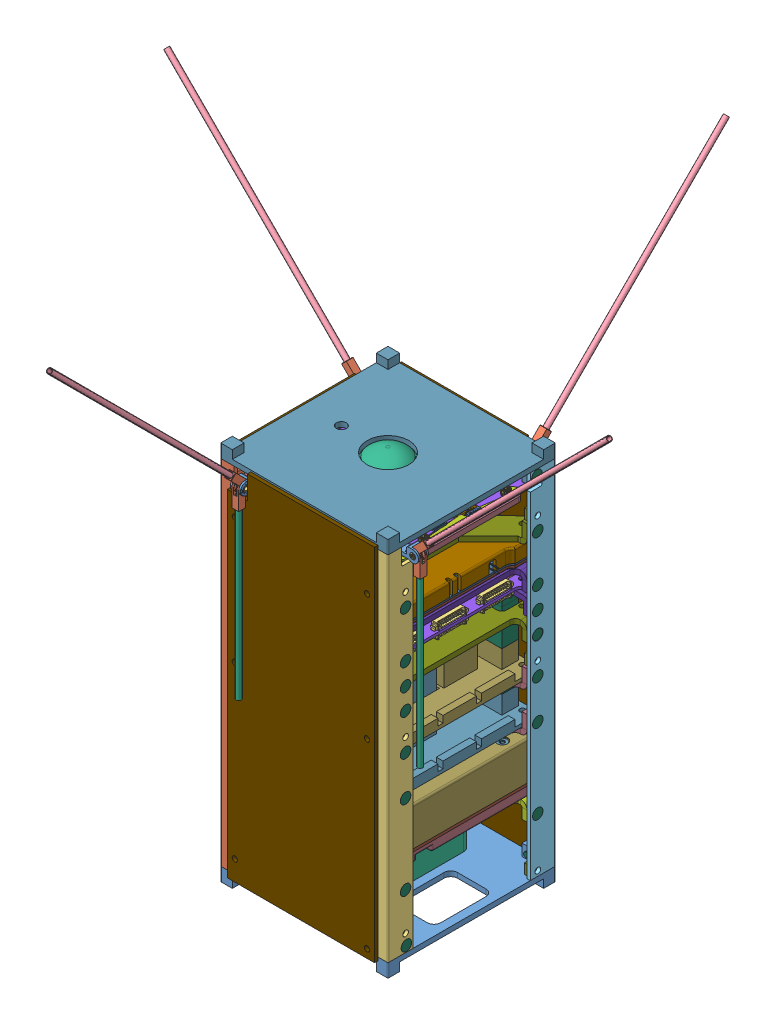
SolidWorks assembly Cubesat, configuration Default. Lengths in mm.
Overall size (336.69 331.47 336.69).
234 component instances, 66 part files, 161 mates.
Components (placement in the parent):
- Cover Plate Bottom-1: Cover Plate Bottom [Default] x (-1 0 0) z (0 0 1) size (100 15 100)
- Rail - Bottom Left-1: Rail - Bottom Left [Default] at (-50 0 50) size (15 211 15)
- Rail - Bottom Right-1: Rail - Bottom Right [Default] at (50 0 50) size (15 211 15)
- Rail - Top Left-1: Rail - Top Left [Default] at (-50 0 -35) size (15 211 15)
- Rail - Top Right-1: Rail - Top Right [Default] at (35 0 -35) size (15 211 15)
- Camera-1: Camera [Default] at (0 36.32 0) x (0 0 1) z (1 0 0) size (50.56 42.32 50.56)
- Camera Plate - 4 tabs - bottom-1: Camera Plate - 4 tabs - bottom [Default] at (0 39.32 0) size (96 10 96)
- EPS1+-1: EPS1+ [Default] at (47.8023 -33.6732 25.0624) x (0 0 -1) z (0 1 0) size (95.9 90.21 30)
  - EPS1+.STEP-1: EPS1+.STEP [Default] at origin size (95.9 90.21 30)
    - ESQ_126_69_G_D.STEP-1: ESQ_126_69_G_D.STEP [Default] at (61.6205 47.1532 90.3532) x (0 -1 0) z (-1 0 0) size (66.55 23.24 5.08)
      - _ESQ_126_69_G_D_socket_2.STEP-1: _ESQ_126_69_G_D_socket_2.STEP [Default] at (-33.274 0 0) size (66.55 8.51 4.95)
      - _ESQ_126_69_G_D_pins_4.STEP-1: _ESQ_126_69_G_D_pins_4.STEP [Default] at origin size (65.79 19.68 4.7)
      - _ESQ_126_69_G_D_LL_bpins_6.STEP-1: _ESQ_126_69_G_D_LL_bpins_6.STEP [Default] at (-33.147 -10.16 0) size (66.04 10.16 5.08)
    - ESQ_126_69_G_D.STEP-2: ESQ_126_69_G_D.STEP [Default] at (66.637 47.1532 90.3532) x (0 1 0) z (1 0 0) size (66.55 23.24 5.08)
      - _ESQ_126_69_G_D_socket_2.STEP-1: _ESQ_126_69_G_D_socket_2.STEP [Default] at (-33.274 0 0) size (66.55 8.51 4.95)
      - _ESQ_126_69_G_D_pins_4.STEP-1: _ESQ_126_69_G_D_pins_4.STEP [Default] at origin size (65.79 19.68 4.7)
      - _ESQ_126_69_G_D_LL_bpins_6.STEP-1: _ESQ_126_69_G_D_LL_bpins_6.STEP [Default] at (-33.147 -10.16 0) size (66.04 10.16 5.08)
    - ES_EPS_Rev1_4_PCB_STEP.STEP-1: ES_EPS_Rev1_4_PCB_STEP.STEP [Default] at (-22.8876 2.7023 80.1932) size (95.9 90.21 13.97)
    - top-cover.STEP-1: top-cover.STEP [Default] at (-22.8876 2.7023 80.1932) size (95.9 90.2 22.8)
    - bottom-cover_Rev1.2.STEP-1: bottom-cover_Rev1.2.STEP [Default] at (25.0624 47.8023 72.9932) size (95.9 90.2 13.5)
    - 965 M3x6 Torx_M3X6mm.STEP-1: 965 M3x6 Torx_M3X6mm.STEP [Default] at (54.8324 9.3023 102.3047) x (-0.142927 0.989733 0) z (0 0 1) size (5.5 5.5 6)
    - 965 M3x6 Torx_M3X6mm.STEP-2: 965 M3x6 Torx_M3X6mm.STEP [Default] at (54.8324 77.0023 102.394) x (0.179192 -0.983814 0) z (0 0 1) size (5.5 5.5 6)
    - TR Fastenings Ltd-M2_5X4mm.STEP-1: TR Fastenings Ltd-M2_5X4mm.STEP [Default] at (-22.8876 68.8523 83.4832) x (0 0.503629 0.86392) z (-1 0 0) size (4.7 4.7 4)
    - TR Fastenings Ltd-M2_5X4mm.STEP-2: TR Fastenings Ltd-M2_5X4mm.STEP [Default] at (-22.8876 26.7523 83.4832) x (0 -0.360323 0.932827) z (-1 0 0) size (4.7 4.7 4)
- Camera-2: Camera [Default] at (0 174.68 0) x (0 0 -1) z (1 0 0) size (50.56 42.32 50.56)
- Camera Plate - 4 tabs - top-1: Camera Plate - 4 tabs - top [Default] at (0 174.68 0) size (96 12 96)
- OBC_EnduroSat-1: OBC_EnduroSat [Default] at (44.1 146.28 47.95) x (0 0 -1) z (0 1 0) size (95 89.38 23.24)
  - OBC_EnduroSat.STEP-1: OBC_EnduroSat.STEP [Default] at origin size (95 89.38 23.24)
    - SD1021117.STEP-1: SD1021117.STEP [Default] at origin size (15.2 14.1 1.88)
      - User_Library-473521001_microSD.STEP-1: User_Library-473521001_microSD.STEP [Default] at (11.4631 39.834 0.9) x (0 -1 0) z (0 0 1) size (14.1 15.2 1.88)
    - P1021117.STEP-1: P1021117.STEP [Default] at origin size (10.15 5.2 3.4)
      - MOLEX_Pico_Blade_532610471.STEP-1: MOLEX_Pico_Blade_532610471.STEP [Default] at (43.8404 79.9325 1.7) size (10.15 5.2 3.4)
        - Open CASCADE STEP translator 6.8 1.14.1.1.STEP-1: Open CASCADE STEP translator 6.8 1.14.1.1.STEP [Default] at origin size (10.15 5.2 3.4)
    - USB1021117.STEP-1: USB1021117.STEP [Default] at origin size (9.9 9.22 5.09)
      - USB_Mini_B_SMT_Horisontal.STEP-1: USB_Mini_B_SMT_Horisontal.STEP [Default] at (43.8628 84.9308 -3.6122) x (1 0 0) z (0 1 0) size (9.9 5.09 9.22)
    - U1021117.STEP-1: U1021117.STEP [Default] at origin size (25.77 25.77 1.57)
      - User_Library-LQFP176-0_5.STEP-1: User_Library-LQFP176-0_5.STEP [Default] at (45.653 34.1752 0.75) x (1 0 0) z (0 0 1) size (25.77 25.77 1.57)
    - PAN6021117.STEP-1: PAN6021117.STEP [Default] at origin size (20.15 5.2 3.5)
      - MOLEX_Pico_Blade_532611271.STEP-1: MOLEX_Pico_Blade_532611271.STEP [Default] at (74.0242 8.708 -1.6) x (-1 0 0) z (0 0 -1) size (20.15 5.2 3.5)
    - PAN5021117.STEP-1: PAN5021117.STEP [Default] at origin size (20.15 5.2 3.5)
      - MOLEX_Pico_Blade_532611271.STEP-1: MOLEX_Pico_Blade_532611271.STEP [Default] at (46.9392 8.708 -1.6) x (-1 0 0) z (0 0 -1) size (20.15 5.2 3.5)
    - PAN4021117.STEP-1: PAN4021117.STEP [Default] at origin size (20.15 5.2 3.5)
      - MOLEX_Pico_Blade_532611271.STEP-1: MOLEX_Pico_Blade_532611271.STEP [Default] at (19.8882 8.708 -1.6) x (-1 0 0) z (0 0 -1) size (20.15 5.2 3.5)
    - PAN3021117.STEP-1: PAN3021117.STEP [Default] at origin size (20.15 5.2 3.5)
      - MOLEX_Pico_Blade_532611271.STEP-1: MOLEX_Pico_Blade_532611271.STEP [Default] at (73.9902 8.708 0) x (1 0 0) z (0 0 1) size (20.15 5.2 3.5)
    - PAN2021117.STEP-1: PAN2021117.STEP [Default] at origin size (20.15 5.2 3.5)
      - MOLEX_Pico_Blade_532611271.STEP-1: MOLEX_Pico_Blade_532611271.STEP [Default] at (46.9392 8.708 0) size (20.15 5.2 3.5)
    - PAN1021117.STEP-1: PAN1021117.STEP [Default] at origin size (20.15 5.2 3.5)
      - MOLEX_Pico_Blade_532611271.STEP-1: MOLEX_Pico_Blade_532611271.STEP [Default] at (19.8882 8.708 0) size (20.15 5.2 3.5)
    - H2021117.STEP-1: H2021117.STEP [Default] at origin size (5.08 66.55 23.24)
      - Samtec-ESQ-126-14-G-D.STEP-1: Samtec-ESQ-126-14-G-D.STEP [Default] at (89.5246 43.45 2.5522) x (-1 0 0) z (0 1 0) size (5.08 23.24 66.55)
    - H1021117.STEP-1: H1021117.STEP [Default] at origin size (5.08 66.55 23.24)
      - Samtec-ESQ-126-14-G-D.STEP-1: Samtec-ESQ-126-14-G-D.STEP [Default] at (84.4446 43.45 2.5522) x (-1 0 0) z (0 1 0) size (5.08 23.24 66.55)
    - J1021117.STEP-1: J1021117.STEP [Default] at origin size (10.55 6.44 2)
      - 5040500491.STEP-1: 5040500491.STEP [Default] at (55.0672 77.863 1) x (1 0 0) z (0 0 1) size (10.55 6.44 2)
        - Open CASCADE STEP translator 6.8 1.245.1.1.STEP-1: Open CASCADE STEP translator 6.8 1.245.1.1.STEP [Default] at origin size (10.55 6.44 2)
    - JP2021117.STEP-1: JP2021117.STEP [Default] at origin size (5.56 20 4.5)
      - Samtec-TLE-110-01-G-DV.STEP-1: Samtec-TLE-110-01-G-DV.STEP [Default] at (68.9102 66.945 2.0874) x (0 1 0) z (1 0 0) size (20 4.5 5.56)
    - JP14021117.STEP-1: JP14021117.STEP [Default] at origin size (5.56 20 4.5)
      - Samtec-TLE-110-01-G-DV.STEP-1: Samtec-TLE-110-01-G-DV.STEP [Default] at (68.8848 66.945 -3.6873) x (0 1 0) z (-1 0 0) size (20 4.5 5.56)
    - JP15021117.STEP-1: JP15021117.STEP [Default] at origin size (20.15 4.2 4.7)
      - User_Library-molex_53398_1271.STEP-1: User_Library-molex_53398_1271.STEP [Default] at (19.1599 50.8269 0) x (1 0 0) z (0 0 1) size (20.15 4.2 4.7)
    - Board021117.STEP-1: Board021117.STEP [Default] at origin size (95 89.38 1.6)
- UHF_comm_type_II-1: UHF_comm_type_II [Default] at (53.7582 76.7976 8.291) x (0 0 -1) z (0 1 0) size (97.88 89.01 26.68)
  - UHF_comm_type_II.STEP-1: UHF_comm_type_II.STEP [Default] at origin size (97.88 89.01 26.68)
    - UHF_BOX.STEP-1: UHF_BOX.STEP [Default] at (-90.205 -23.549 76.8824) size (95 89 8.01)
    - UHF_PCB_STEP.STEP-1: UHF_PCB_STEP.STEP [Default] at (-39.659 9.6582 83.8824) size (97.88 89.01 26.68)
    - UHF_BOX-bottom-part(nif).STEP-1: UHF_BOX-bottom-part(nif).STEP [Default] at (-24.9069 125.9519 81.8824) x (1 0 0) z (0 -1 0) size (95 2.01 89)
- Custom Board 1-1: Custom Board 1 [Default] at (0 99.589 0) size (88 32 93.7)
- Custom Board 1 Plate-1: Custom Board 1 Plate [Default] at (0 99.589 0) size (96 12 93.7)
- Custom Board 2-1: Custom Board 2 [Default] at (0 75.989 0) size (88 62 93.7)
- PC104 Connector-1: PC104 Connector [Default] at (-32.6269 65.189 -34.0211) x (1 0 0) z (0 0 1) size (66.55 22.99 10.03)
- Custom Board 1 Plate-2: Custom Board 1 Plate [Default] at (0 75.989 0) size (96 12 93.7)
- PC104 Connector-2: PC104 Connector [Default] at (-32.627 88.789 -34.051) size (66.55 22.99 10.03)
- PC104 Connector-3: PC104 Connector [Default] at (-32.627 133.989 -34.112) size (66.55 22.99 10.03)
- PC104 Connector-4: PC104 Connector [Default] at (-32.627 112.389 -34.112) size (66.55 22.99 10.03)
- PC104 Connector-5: PC104 Connector [Default] at (-32.627 123.189 -34.112) size (66.55 22.99 10.03)
- Engraving plate-1: Engraving plate [Default] at (0 131.989 0) size (96 10 93.7)
- OBC Board Plate-1: OBC Board Plate [Default] at (0 144.68 0) size (96 10 93.7)
- Engraving-1: Engraving [Default] at (0 131.989 0) x (-1 0 0) z (0 0 -1) size (55 5 55)
- gs-3dcad-nanocom-ant430-2u3u-deployed-4-1: gs-3dcad-nanocom-ant430-2u3u-deployed-4 [Default] at (-41.1027 203 -16.9694) x (0 0 1) z (0 1 0) size (336.69 336.69 122.72)
  - antenna-assembly-top-2U-4.0_ant430-2U-4(Deployed)-1-1: antenna-assembly-top-2U-4.0_ant430-2U-4(Deployed)-1 [Default] at (48.1694 3.1027 0) x (1 0 0) z (0 -1 0) size (137.15 122.72 6)
    - antenna-bracket-top-2_ant430-2U-4-1: antenna-bracket-top-2_ant430-2U-4 [Default] at (17.9301 -0.951 -3) size (25 7 6)
    - antenna-fork-top-1_ant430-2U-4-1: antenna-fork-top-1_ant430-2U-4 [Default] at (15.39 -4.0676 -3) x (-0.707107 -0.707107 0) z (0 0 -1) size (14.46 7 4)
    - antenna-fork-top-bush_ant430-2U-4-1: antenna-fork-top-bush_ant430-2U-4 [Default] at (26.2784 -6.4189 -6) x (0.730043 -0.683401 0) z (0 0 1) size (3.5 3.5 6)
    - antenna-170_ant430-2U-4-1: antenna-170_ant430-2U-4 [Default] at (22.8888 6.2101 -3) x (-0.041594 0.041594 -0.998268) z (0.707107 0.707107 0) size (3 3 160)
    - ISO 7046-1 - M2,5 x 6 - 4.8 - HDIN EN ISO_ant430-2U-4-1: ISO 7046-1 - M2,5 x 6 - 4.8 - HDIN EN ISO_ant430-2U-4 [Default] at (9.3 1.612 -3) x (0 -1 0) z (0.947379 0 0.320115) size (2.81 4.7 4.7)
    - ISO 7046-1 - M2,5 x 6 - 4.8 - HDIN EN ISO_1_ant430-2U-4-1: ISO 7046-1 - M2,5 x 6 - 4.8 - HDIN EN ISO_1_ant430-2U-4 [Default] at (3.3 1.612 -3) x (0 -1 0) z (0 0 1) size (2.81 4.7 4.7)
  - antenna-assembly-top-2U-4.0_ant430-2U-4(Deployed)-2-1: antenna-assembly-top-2U-4.0_ant430-2U-4(Deployed)-2 [Default] at (54.9694 72.3027 0) x (0 1 0) z (1 0 0) size (137.15 122.72 6)
    - antenna-bracket-top-2_ant430-2U-4-1: antenna-bracket-top-2_ant430-2U-4 [Default] at (17.9301 -0.951 -3) size (25 7 6)
    - antenna-fork-top-1_ant430-2U-4-1: antenna-fork-top-1_ant430-2U-4 [Default] at (15.39 -4.0676 -3) x (-0.707107 -0.707107 0) z (0 0 -1) size (14.46 7 4)
    - antenna-fork-top-bush_ant430-2U-4-1: antenna-fork-top-bush_ant430-2U-4 [Default] at (26.2784 -6.4189 -6) x (0.730043 -0.683401 0) z (0 0 1) size (3.5 3.5 6)
    - antenna-170_ant430-2U-4-1: antenna-170_ant430-2U-4 [Default] at (22.8888 6.2101 -3) x (-0.041594 0.041594 -0.998268) z (0.707107 0.707107 0) size (3 3 160)
    - ISO 7046-1 - M2,5 x 6 - 4.8 - HDIN EN ISO_ant430-2U-4-1: ISO 7046-1 - M2,5 x 6 - 4.8 - HDIN EN ISO_ant430-2U-4 [Default] at (9.3 1.612 -3) x (0 -1 0) z (0.947379 0 0.320115) size (2.81 4.7 4.7)
    - ISO 7046-1 - M2,5 x 6 - 4.8 - HDIN EN ISO_1_ant430-2U-4-1: ISO 7046-1 - M2,5 x 6 - 4.8 - HDIN EN ISO_1_ant430-2U-4 [Default] at (3.3 1.612 -3) x (0 -1 0) z (0 0 1) size (2.81 4.7 4.7)
  - antenna-assembly-top-2U-4.0_ant430-2U-4(Deployed)-3-1: antenna-assembly-top-2U-4.0_ant430-2U-4(Deployed)-3 [Default] at (-21.0306 9.9027 0) x (0 -1 0) z (-1 0 0) size (137.15 122.72 6)
    - antenna-bracket-top-2_ant430-2U-4-1: antenna-bracket-top-2_ant430-2U-4 [Default] at (17.9301 -0.951 -3) size (25 7 6)
    - antenna-fork-top-1_ant430-2U-4-1: antenna-fork-top-1_ant430-2U-4 [Default] at (15.39 -4.0676 -3) x (-0.707107 -0.707107 0) z (0 0 -1) size (14.46 7 4)
    - antenna-fork-top-bush_ant430-2U-4-1: antenna-fork-top-bush_ant430-2U-4 [Default] at (26.2784 -6.4189 -6) x (0.730043 -0.683401 0) z (0 0 1) size (3.5 3.5 6)
    - antenna-170_ant430-2U-4-1: antenna-170_ant430-2U-4 [Default] at (22.8888 6.2101 -3) x (-0.041594 0.041594 -0.998268) z (0.707107 0.707107 0) size (3 3 160)
    - ISO 7046-1 - M2,5 x 6 - 4.8 - HDIN EN ISO_ant430-2U-4-1: ISO 7046-1 - M2,5 x 6 - 4.8 - HDIN EN ISO_ant430-2U-4 [Default] at (9.3 1.612 -3) x (0 -1 0) z (0.947379 0 0.320115) size (2.81 4.7 4.7)
    - ISO 7046-1 - M2,5 x 6 - 4.8 - HDIN EN ISO_1_ant430-2U-4-1: ISO 7046-1 - M2,5 x 6 - 4.8 - HDIN EN ISO_1_ant430-2U-4 [Default] at (3.3 1.612 -3) x (0 -1 0) z (0 0 1) size (2.81 4.7 4.7)
  - antenna-assembly-top-2U-4.0_ant430-2U-4(Deployed)-4-1: antenna-assembly-top-2U-4.0_ant430-2U-4(Deployed)-4 [Default] at (-14.2306 79.1027 0) x (-1 0 0) z (0 1 0) size (137.15 122.72 6)
    - antenna-bracket-top-2_ant430-2U-4-1: antenna-bracket-top-2_ant430-2U-4 [Default] at (17.9301 -0.951 -3) size (25 7 6)
    - antenna-fork-top-1_ant430-2U-4-1: antenna-fork-top-1_ant430-2U-4 [Default] at (15.39 -4.0676 -3) x (-0.707107 -0.707107 0) z (0 0 -1) size (14.46 7 4)
    - antenna-fork-top-bush_ant430-2U-4-1: antenna-fork-top-bush_ant430-2U-4 [Default] at (26.2784 -6.4189 -6) x (0.730043 -0.683401 0) z (0 0 1) size (3.5 3.5 6)
    - antenna-170_ant430-2U-4-1: antenna-170_ant430-2U-4 [Default] at (22.8888 6.2101 -3) x (-0.041594 0.041594 -0.998268) z (0.707107 0.707107 0) size (3 3 160)
    - ISO 7046-1 - M2,5 x 6 - 4.8 - HDIN EN ISO_ant430-2U-4-1: ISO 7046-1 - M2,5 x 6 - 4.8 - HDIN EN ISO_ant430-2U-4 [Default] at (9.3 1.612 -3) x (0 -1 0) z (0.947379 0 0.320115) size (2.81 4.7 4.7)
    - ISO 7046-1 - M2,5 x 6 - 4.8 - HDIN EN ISO_1_ant430-2U-4-1: ISO 7046-1 - M2,5 x 6 - 4.8 - HDIN EN ISO_1_ant430-2U-4 [Default] at (3.3 1.612 -3) x (0 -1 0) z (0 0 1) size (2.81 4.7 4.7)
  - J1_ant430-2U-4-1: J1_ant430-2U-4 [Default] at (3.9323 135.2339 -0.0972) x (-0.00113 -0.999999 0) z (0 0 1) size (9.3 6.7 5)
    - MCX-J-P-X-ST-EM1_ant430-2U-4-1: MCX-J-P-X-ST-EM1_ant430-2U-4 [Default] at (55.475 16.8643 0.4627) x (0 1 0) z (0 0 -1) size (6.7 9.3 5)
  - panel-top_ant430-2U-4-1: panel-top_ant430-2U-4 [Default] at origin size (98 98 1)
  - hirose-ufl_ant430-2U-4-1: hirose-ufl_ant430-2U-4 [Default] at (-12.7135 4.105 -3.7628) x (0 1 0) z (1 0 0) size (3 1.25 3)
  - hirose-ufl_ant430-2U-4-2: hirose-ufl_ant430-2U-4 [Default] at (55.4593 87.5833 -3.7628) x (1 0 0) z (0 -1 0) size (3 1.25 3)
  - hirose-ufl_ant430-2U-4-3: hirose-ufl_ant430-2U-4 [Default] at (63.2738 2.5816 -3.7628) x (0 -1 0) z (-1 0 0) size (3 1.25 3)
  - hirose-ufl_ant430-2U-4-4: hirose-ufl_ant430-2U-4 [Default] at (-20.4856 70.6906 -3.7628) x (1 0 0) z (0 -1 0) size (3 1.25 3)
  - qba07_ant430-2U-4-1: qba07_ant430-2U-4 [Default] at (23.1375 84.762 0.07) x (1 -0.000453 0) z (0 0 1) size (7.5 6.3 1.1)
  - qba07_ant430-2U-4-2: qba07_ant430-2U-4 [Default] at (41.0317 82.0693 0.07) x (1 0.000095 0) z (0 0 1) size (7.5 6.3 1.1)
  - qba07_ant430-2U-4-3: qba07_ant430-2U-4 [Default] at (33.3017 -0.4434 0.07) x (1 -0.000112 0) z (0 0 1) size (7.5 6.3 1.1)
  - R0603_ant430-2U-4-1: R0603_ant430-2U-4 [Default] at (30.2037 57.3599 0.4127) x (0.000486 1 0) z (0 0 -1) size (0.88 2.08 0.4)
  - R0603_ant430-2U-4-2: R0603_ant430-2U-4 [Default] at (-21.9072 52.5823 0.4127) x (0.00281 0.999996 0) z (0 0 -1) size (0.88 2.08 0.4)
  - R0603_ant430-2U-4-3: R0603_ant430-2U-4 [Default] at (11.8469 60.1356 0.4127) x (0.014872 0.999889 0) z (0 0 -1) size (0.88 2.08 0.4)
  - R0603_ant430-2U-4-4: R0603_ant430-2U-4 [Default] at (54.4868 -8.4911 0.4127) x (-0.008918 0.99996 0) z (0 0 -1) size (0.88 2.08 0.4)
  - R0603_ant430-2U-4-5: R0603_ant430-2U-4 [Default] at (-32.7203 4.2504 0.4127) x (1 0 0) z (0 0 -1) size (0.88 2.08 0.4)
  - R0603_ant430-2U-4-6: R0603_ant430-2U-4 [Default] at (-2.4272 2.3806 0.4127) x (1 0 0) z (0 0 -1) size (0.88 2.08 0.4)
  - R0603_ant430-2U-4-7: R0603_ant430-2U-4 [Default] at (28.1277 79.0766 0.4127) x (1 0 0) z (0 0 -1) size (0.88 2.08 0.4)
  - 2.5x4.5x3.0mm-spacer_ant430-2U-4-1: 2.5x4.5x3.0mm-spacer_ant430-2U-4 [Default] at (41.6694 86.9027 3) x (1 0 0) z (0 0 -1) size (4.5 4.5 3)
  - 2.5x4.5x3.0mm-spacer_ant430-2U-4-2: 2.5x4.5x3.0mm-spacer_ant430-2U-4 [Default] at (-7.7306 -4.6973 3) x (1 0 0) z (0 0 -1) size (4.5 4.5 3)
  - 2.5x4.5x3.0mm-spacer_ant430-2U-4-3: 2.5x4.5x3.0mm-spacer_ant430-2U-4 [Default] at (-7.7306 86.9027 3) x (1 0 0) z (0 0 -1) size (4.5 4.5 3)
  - 2.5x4.5x3.0mm-spacer_ant430-2U-4-4: 2.5x4.5x3.0mm-spacer_ant430-2U-4 [Default] at (41.6694 -4.6973 3) x (1 0 0) z (0 0 -1) size (4.5 4.5 3)
- Antenna Plate-1: Antenna Plate [Default] at (0 202 0) x (-1 0 0) z (0 0 -1) size (100 10 96)
- Cover Plate Top-2: Cover Plate Top [Default] at (0 211 0) size (100 15 100)
- M3 Flathead-1: M3 Flathead [Default] at (-50 150.8117 39.5) x (0 -1 0) z (0 0 1) size (6.3 6.45 6.3)
- M3 Flathead-2: M3 Flathead [Default] at (-50 79.8607 39.5) x (0 -1 0) z (0 0 1) size (6.3 6.45 6.3)
- M3 Flathead-3: M3 Flathead [Default] at (-50 178.5483 39.5) x (0 -1 0) z (0 0 1) size (6.3 6.45 6.3)
- M3 Flathead-4: M3 Flathead [Default] at (-49.8242 150.8117 -39.5) x (0 -1 0) z (0 0 1) size (6.3 6.45 6.3)
- M3 Flathead-5: M3 Flathead [Default] at (-50 103.4607 39.5) x (0 -1 0) z (0 0 1) size (6.3 6.45 6.3)
- M3 Flathead-6: M3 Flathead [Default] at (-50 178.5483 -39.5) x (0 -1 0) z (0 0 1) size (6.3 6.45 6.3)
- M3 Flathead-7: M3 Flathead [Default] at (-50 32.4507 39.5) x (0 -1 0) z (0 0 1) size (6.3 6.45 6.3)
- M3 Flathead-8: M3 Flathead [Default] at (-50 125.1207 39.5) x (0 -1 0) z (0 0 1) size (6.3 6.45 6.3)
- M3 Flathead-9: M3 Flathead [Default] at (-50 103.4607 -39.5) x (0 -1 0) z (0 0 1) size (6.3 6.45 6.3)
- M3 Flathead-10: M3 Flathead [Default] at (-50 79.8607 -39.5) x (0 -1 0) z (0 0 1) size (6.3 6.45 6.3)
- M3 Flathead-11: M3 Flathead [Default] at (-50 125.1207 -39.5) x (0 -1 0) z (0 0 1) size (6.3 6.45 6.3)
- M3 Flathead-12: M3 Flathead [Default] at (-50 137.8117 -39.5) x (0 -1 0) z (0 0 1) size (6.3 6.45 6.3)
- M3 Flathead-13: M3 Flathead [Default] at (-50 32.4507 -39.5) x (0 -1 0) z (0 0 1) size (6.3 6.45 6.3)
- M3 Flathead-14: M3 Flathead [Default] at (50 178.5483 39.5) x (0 1 0) z (0 0 1) size (6.3 6.45 6.3)
- M3 Flathead-15: M3 Flathead [Default] at (50 178.5483 -39.5) x (0 1 0) z (0 0 1) size (6.3 6.45 6.3)
- M3 Flathead-16: M3 Flathead [Default] at (50 150.8117 39.5) x (0 1 0) z (0 0 1) size (6.3 6.45 6.3)
- M3 Flathead-17: M3 Flathead [Default] at (50 150.8117 -39.5) x (0 1 0) z (0 0 1) size (6.3 6.45 6.3)
- M3 Flathead-18: M3 Flathead [Default] at (50 137.8117 39.5) x (0 1 0) z (0 0 1) size (6.3 6.45 6.3)
- M3 Flathead-19: M3 Flathead [Default] at (50 137.8117 -39.5) x (0 1 0) z (0 0 1) size (6.3 6.45 6.3)
- M3 Flathead-20: M3 Flathead [Default] at (50 125.1207 39.5) x (0 1 0) z (0 0 1) size (6.3 6.45 6.3)
- M3 Flathead-21: M3 Flathead [Default] at (49.8242 125.1207 -39.5) x (0 1 0) z (0 0 1) size (6.3 6.45 6.3)
- M3 Flathead-22: M3 Flathead [Default] at (50 103.5207 39.5) x (0 1 0) z (0 0 1) size (6.3 6.45 6.3)
- M3 Flathead-23: M3 Flathead [Default] at (50 103.4607 -39.5) x (0 1 0) z (0 0 1) size (6.3 6.45 6.3)
- M3 Flathead-24: M3 Flathead [Default] at (50 79.9207 39.5) x (0 0.454172 0.890914) z (0 -0.890914 0.454172) size (6.3 6.45 6.3)
- M3 Flathead-25: M3 Flathead [Default] at (50 32.5107 39.5) x (0 1 0) z (0 0 1) size (6.3 6.45 6.3)
- M3 Flathead-26: M3 Flathead [Default] at (50 79.8607 -39.5) x (0 1 0) z (0 0 1) size (6.3 6.45 6.3)
- M3 Flathead-27: M3 Flathead [Default] at (50 32.4507 -39.5) x (0 0.965001 -0.262245) z (0 0.262245 0.965001) size (6.3 6.45 6.3)
- M3 Flathead-28: M3 Flathead [Default] at (-39 207.5 -50) x (1 0 0) z (0 -1 0) size (6.3 6.45 6.3)
- M3 Flathead-29: M3 Flathead [Default] at (-50 207.5 39) x (0 -1 0) z (0 0 1) size (6.3 6.45 6.3)
- M3 Flathead-30: M3 Flathead [Default] at (50 207.5 -39) x (0 1 0) z (0 0 1) size (6.3 6.45 6.3)
- M3 Flathead-31: M3 Flathead [Default] at (39 207.5 50) x (1 0 0) z (0 1 0) size (6.3 6.45 6.3)
- M3 Flathead-32: M3 Flathead [Default] at (-39 3.5 50) x (1 0 0) z (0 1 0) size (6.3 6.45 6.3)
- M3 Flathead-33: M3 Flathead [Default] at (50 3.5 39) x (0 1 0) z (0 0 1) size (6.3 6.45 6.3)
- M3 Flathead-34: M3 Flathead [Default] at (39 3.5 -50) x (1 0 0) z (0 -1 0) size (6.3 6.45 6.3)
- M3 Flathead-35: M3 Flathead [Default] at (-50 3.5 -39) x (0 -1 0) z (0 0 1) size (6.3 6.45 6.3)
- M3 Flathead-36: M3 Flathead [Default] at (-50 137.8117 39.5) x (0 -1 0) z (0 0 1) size (6.3 6.45 6.3)
- M3 Square Nut-17: M3 Square Nut [Default] at (-45 7 -36.5) x (0 1 0) z (-1 0 0) size (6 6 3)
- M3 Square Nut-18: M3 Square Nut [Default] at (-45 114.589 -36.5) x (0 0 -1) z (-1 0 0) size (6 6 3)
- M3 Square Nut-20: M3 Square Nut [Default] at (-45 189.68 -42.5) x (0 -1 0) z (-1 0 0) size (6 6 3)
- M3 Square Nut-21: M3 Square Nut [Default] at (-48 6 36.5) x (0 0 1) z (1 0 0) size (6 6 3)
- M3 Square Nut-22: M3 Square Nut [Default] at (-45 114.589 42.5) x (0 0 -1) z (-1 0 0) size (6 6 3)
- M3 Square Nut-24: M3 Square Nut [Default] at (-48 183.68 36.5) x (0 1 0) z (1 0 0) size (6 6 3)
- M3 Square Nut-25: M3 Square Nut [Default] at (45 0 -36.5) x (0 0 -1) z (1 0 0) size (6 6 3)
- M3 Square Nut-26: M3 Square Nut [Default] at (45 114.589 -36.5) x (0 -1 0) z (1 0 0) size (6 6 3)
- M3 Square Nut-28: M3 Square Nut [Default] at (45 183.68 -36.5) x (0 0 -1) z (1 0 0) size (6 6 3)
- M3 Square Nut-29: M3 Square Nut [Default] at (45 13 42.5) x (0 -1 0) z (1 0 0) size (6 6 3)
- M3 Square Nut-30: M3 Square Nut [Default] at (45 114.589 36.5) x (0 0 1) z (1 0 0) size (6 6 3)
- M3 Square Nut-32: M3 Square Nut [Default] at (45 183.68 42.5) x (0 0 -1) z (1 0 0) size (6 6 3)
- Custom Plate - tabs down-1: Custom Plate - tabs down [Default] at (0 157.68 0) size (96 10 93.7)
- Solar panel plate-2: Solar panel plate [Default] at (-44 -2 50) size (88 215 2)
- Solar panel plate-3: Solar panel plate [Default] at (44 -2 -50) x (-1 0 0) z (0 0 -1) size (88 215 2)
- Solar panel plate-4: Solar panel plate [Default] at (-50 -2 -44) x (0 0 1) z (-1 0 0) size (88 215 2)
- Solar panel plate-5: Solar panel plate [Default] at (50 -2 44) x (0 0 -1) z (1 0 0) size (88 215 2) (hidden)
- gs-3dcad-nanocom-ant430-1u-stowed-4-1: gs-3dcad-nanocom-ant430-1u-stowed-4 [Default] at (41.1027 203 16.9694) x (0 0 -1) z (0 1 0) size (112.64 112.64 113.03)
  - antenna-assembly-top-2U-4.0_ant430-1U-4(Default - Stowed)-1: antenna-assembly-top-2U-4.0_ant430-1U-4(Default - Stowed) [Default] at (66.0994 6.1027 -0.951) x (1 0 0) z (0 -1 0) size (25.12 112.96 6)
    - antenna-bracket-top-2_ant430-1U-4-1: antenna-bracket-top-2_ant430-1U-4 [Default] at origin size (25 7 6)
    - antenna-fork-top-1_ant430-1U-4-1: antenna-fork-top-1_ant430-1U-4 [Default] at (3.1049 12.7569 0) x (0 1 0) z (0 0 -1) size (14.46 7 4)
    - antenna-fork-top-bush_ant430-1U-4-1: antenna-fork-top-bush_ant430-1U-4 [Default] at (8.045 -5.6205 -3) x (0.707107 -0.707107 0) z (0 0 1) size (3.5 3.5 6)
    - ISO 7046-1 - M2,5 x 6 - 4.8 - HDIN EN ISO_ant430-1U-4-1: ISO 7046-1 - M2,5 x 6 - 4.8 - HDIN EN ISO_ant430-1U-4 [Default] at (-8.6301 2.563 0) x (0 -1 0) z (0.947379 0 0.320115) size (2.81 4.7 4.7)
    - ISO 7046-1 - M2,5 x 6 - 4.8 - HDIN EN ISO_1_ant430-1U-4-1: ISO 7046-1 - M2,5 x 6 - 4.8 - HDIN EN ISO_1_ant430-1U-4 [Default] at (-14.6301 2.563 0) x (0 -1 0) z (0 0 1) size (2.81 4.7 4.7)
    - Antenna_AluRod(3mm x 106)-1: Antenna_AluRod(3mm x 106) [Default] at (5.0699 0.1869 0) x (0.707107 0 -0.707107) z (0 -1 0) size (3 3 106)
  - antenna-assembly-top-2U-4.0_ant430-1U-4(Default - Stowed)-1-1: antenna-assembly-top-2U-4.0_ant430-1U-4(Default - Stowed)-1 [Default] at (51.9694 90.2328 -0.951) x (0 1 0) z (1 0 0) size (25.12 112.96 6)
    - antenna-bracket-top-2_ant430-1U-4-1: antenna-bracket-top-2_ant430-1U-4 [Default] at origin size (25 7 6)
    - antenna-fork-top-1_ant430-1U-4-1: antenna-fork-top-1_ant430-1U-4 [Default] at (3.1049 12.7569 0) x (0 1 0) z (0 0 -1) size (14.46 7 4)
    - antenna-fork-top-bush_ant430-1U-4-1: antenna-fork-top-bush_ant430-1U-4 [Default] at (8.045 -5.6205 -3) x (0.707107 -0.707107 0) z (0 0 1) size (3.5 3.5 6)
    - ISO 7046-1 - M2,5 x 6 - 4.8 - HDIN EN ISO_ant430-1U-4-1: ISO 7046-1 - M2,5 x 6 - 4.8 - HDIN EN ISO_ant430-1U-4 [Default] at (-8.6301 2.563 0) x (0 -1 0) z (0.947379 0 0.320115) size (2.81 4.7 4.7)
    - ISO 7046-1 - M2,5 x 6 - 4.8 - HDIN EN ISO_1_ant430-1U-4-1: ISO 7046-1 - M2,5 x 6 - 4.8 - HDIN EN ISO_1_ant430-1U-4 [Default] at (-14.6301 2.563 0) x (0 -1 0) z (0 0 1) size (2.81 4.7 4.7)
    - Antenna_AluRod(3mm x 106)-1: Antenna_AluRod(3mm x 106) [Default] at (5.0699 0.1869 0) x (0.707107 0 -0.707107) z (0 -1 0) size (3 3 106)
  - antenna-assembly-top-2U-4.0_ant430-1U-4(Default - Stowed)-2-1: antenna-assembly-top-2U-4.0_ant430-1U-4(Default - Stowed)-2 [Default] at (-18.0306 -8.0274 -0.951) x (0 -1 0) z (-1 0 0) size (25.12 112.96 6)
    - antenna-bracket-top-2_ant430-1U-4-1: antenna-bracket-top-2_ant430-1U-4 [Default] at origin size (25 7 6)
    - antenna-fork-top-1_ant430-1U-4-1: antenna-fork-top-1_ant430-1U-4 [Default] at (3.1049 12.7569 0) x (0 1 0) z (0 0 -1) size (14.46 7 4)
    - antenna-fork-top-bush_ant430-1U-4-1: antenna-fork-top-bush_ant430-1U-4 [Default] at (8.045 -5.6205 -3) x (0.707107 -0.707107 0) z (0 0 1) size (3.5 3.5 6)
    - ISO 7046-1 - M2,5 x 6 - 4.8 - HDIN EN ISO_ant430-1U-4-1: ISO 7046-1 - M2,5 x 6 - 4.8 - HDIN EN ISO_ant430-1U-4 [Default] at (-8.6301 2.563 0) x (0 -1 0) z (0.947379 0 0.320115) size (2.81 4.7 4.7)
    - ISO 7046-1 - M2,5 x 6 - 4.8 - HDIN EN ISO_1_ant430-1U-4-1: ISO 7046-1 - M2,5 x 6 - 4.8 - HDIN EN ISO_1_ant430-1U-4 [Default] at (-14.6301 2.563 0) x (0 -1 0) z (0 0 1) size (2.81 4.7 4.7)
    - Antenna_AluRod(3mm x 106)-1: Antenna_AluRod(3mm x 106) [Default] at (5.0699 0.1869 0) x (0.707107 0 -0.707107) z (0 -1 0) size (3 3 106)
  - antenna-assembly-top-2U-4.0_ant430-1U-4(Default - Stowed)-3-1: antenna-assembly-top-2U-4.0_ant430-1U-4(Default - Stowed)-3 [Default] at (-32.1607 76.1027 -0.881) x (-1 0 0) z (0 1 0) size (25.12 112.96 6)
    - antenna-bracket-top-2_ant430-1U-4-1: antenna-bracket-top-2_ant430-1U-4 [Default] at origin size (25 7 6)
    - antenna-fork-top-1_ant430-1U-4-1: antenna-fork-top-1_ant430-1U-4 [Default] at (3.1049 12.7569 0) x (0 1 0) z (0 0 -1) size (14.46 7 4)
    - antenna-fork-top-bush_ant430-1U-4-1: antenna-fork-top-bush_ant430-1U-4 [Default] at (8.045 -5.6205 -3) x (0.707107 -0.707107 0) z (0 0 1) size (3.5 3.5 6)
    - ISO 7046-1 - M2,5 x 6 - 4.8 - HDIN EN ISO_ant430-1U-4-1: ISO 7046-1 - M2,5 x 6 - 4.8 - HDIN EN ISO_ant430-1U-4 [Default] at (-8.6301 2.563 0) x (0 -1 0) z (0.947379 0 0.320115) size (2.81 4.7 4.7)
    - ISO 7046-1 - M2,5 x 6 - 4.8 - HDIN EN ISO_1_ant430-1U-4-1: ISO 7046-1 - M2,5 x 6 - 4.8 - HDIN EN ISO_1_ant430-1U-4 [Default] at (-14.6301 2.563 0) x (0 -1 0) z (0 0 1) size (2.81 4.7 4.7)
    - Antenna_AluRod(3mm x 106)-1: Antenna_AluRod(3mm x 106) [Default] at (5.0699 0.1869 0) x (0.707107 0 -0.707107) z (0 -1 0) size (3 3 106)
  - panel-top_ant430-1U-4-1: panel-top_ant430-1U-4 [Default] at origin size (98 98 1)
  - hirose-ufl_ant430-1U-4-1: hirose-ufl_ant430-1U-4 [Default] at (55.4593 87.5833 -3.7628) x (1 0 0) z (0 -1 0) size (3 1.25 3)
  - hirose-ufl_ant430-1U-4-2: hirose-ufl_ant430-1U-4 [Default] at (63.2738 2.5816 -3.7628) x (0 -1 0) z (-1 0 0) size (3 1.25 3)
  - hirose-ufl_ant430-1U-4-3: hirose-ufl_ant430-1U-4 [Default] at (-20.4856 70.6906 -3.7628) x (1 0 0) z (0 -1 0) size (3 1.25 3)
  - hirose-ufl_ant430-1U-4-4: hirose-ufl_ant430-1U-4 [Default] at (-12.7135 4.105 -3.7628) x (0 1 0) z (1 0 0) size (3 1.25 3)
  - qba07_ant430-1U-4-1: qba07_ant430-1U-4 [Default] at (23.1375 84.762 0.07) x (1 -0.000453 0) z (0 0 1) size (7.5 6.3 1.1)
  - qba07_ant430-1U-4-2: qba07_ant430-1U-4 [Default] at (33.3017 -0.4434 0.07) x (1 -0.000112 0) z (0 0 1) size (7.5 6.3 1.1)
  - qba07_ant430-1U-4-3: qba07_ant430-1U-4 [Default] at (41.0317 82.0693 0.07) x (1 0.000095 0) z (0 0 1) size (7.5 6.3 1.1)
  - ssmcx-flat_ant430-1U-4-1: ssmcx-flat_ant430-1U-4 [Default] at (22.3251 74.715 -0.86) x (-1 0 0) z (0 1 0) size (3.91 2.3 7.72)
  - R0603_ant430-1U-4-1: R0603_ant430-1U-4 [Default] at (11.8469 60.1356 0.4127) x (0.014872 0.999889 0) z (0 0 -1) size (0.88 2.08 0.4)
  - R0603_ant430-1U-4-2: R0603_ant430-1U-4 [Default] at (28.1277 79.0766 0.4127) x (1 0 0) z (0 0 -1) size (0.88 2.08 0.4)
  - R0603_ant430-1U-4-3: R0603_ant430-1U-4 [Default] at (-2.4272 2.3806 0.4127) x (1 0 0) z (0 0 -1) size (0.88 2.08 0.4)
  - R0603_ant430-1U-4-4: R0603_ant430-1U-4 [Default] at (-32.7203 4.2504 0.4127) x (1 0 0) z (0 0 -1) size (0.88 2.08 0.4)
  - R0603_ant430-1U-4-5: R0603_ant430-1U-4 [Default] at (-21.9072 52.5823 0.4127) x (0.00281 0.999996 0) z (0 0 -1) size (0.88 2.08 0.4)
  - R0603_ant430-1U-4-6: R0603_ant430-1U-4 [Default] at (54.4868 -8.4911 0.4127) x (-0.008918 0.99996 0) z (0 0 -1) size (0.88 2.08 0.4)
  - R0603_ant430-1U-4-7: R0603_ant430-1U-4 [Default] at (30.2037 57.3599 0.4127) x (0.000486 1 0) z (0 0 -1) size (0.88 2.08 0.4)
  - 2.5x4.5x3.0mm-spacer_ant430-1U-4-1: 2.5x4.5x3.0mm-spacer_ant430-1U-4 [Default] at (41.6694 86.9027 3) x (1 0 0) z (0 0 -1) size (4.5 4.5 3)
  - 2.5x4.5x3.0mm-spacer_ant430-1U-4-2: 2.5x4.5x3.0mm-spacer_ant430-1U-4 [Default] at (-7.7306 -4.6973 3) x (1 0 0) z (0 0 -1) size (4.5 4.5 3)
  - 2.5x4.5x3.0mm-spacer_ant430-1U-4-3: 2.5x4.5x3.0mm-spacer_ant430-1U-4 [Default] at (-7.7306 86.9027 3) x (1 0 0) z (0 0 -1) size (4.5 4.5 3)
  - 2.5x4.5x3.0mm-spacer_ant430-1U-4-4: 2.5x4.5x3.0mm-spacer_ant430-1U-4 [Default] at (41.6694 -4.6973 3) x (1 0 0) z (0 0 -1) size (4.5 4.5 3)
